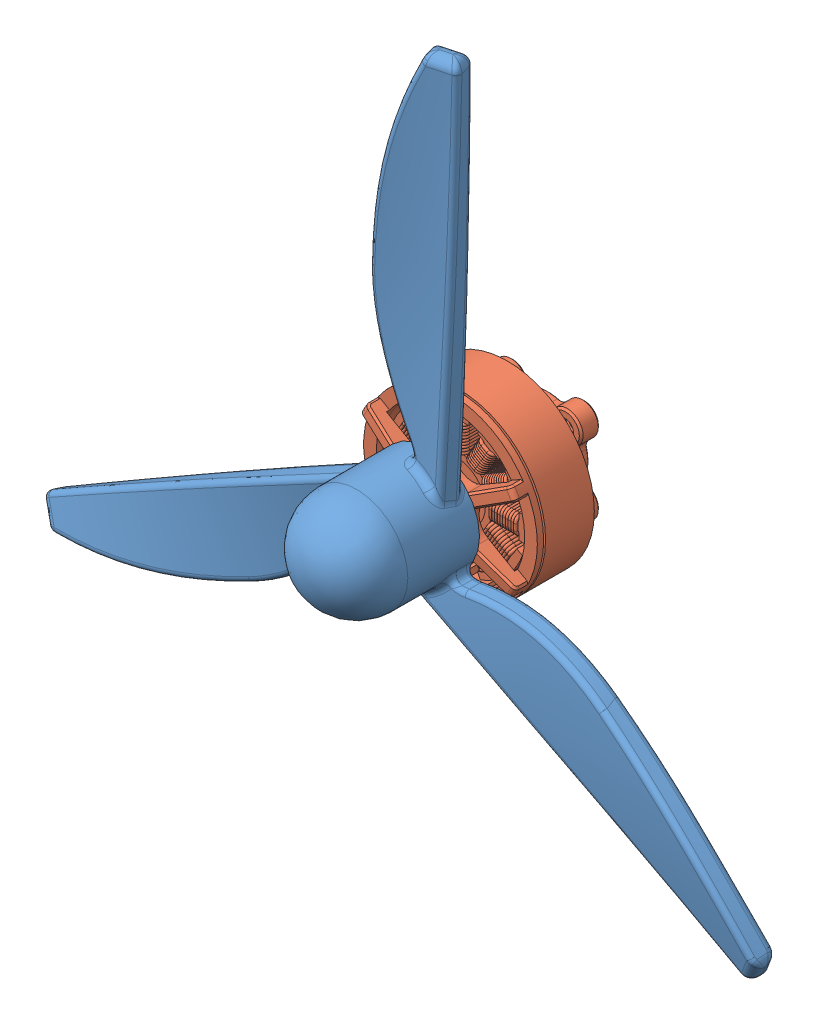
SolidWorks assembly 装配体3, configuration 默认. Lengths in mm.
Overall size (116.58 102.47 38.52).
2 component instances, 2 part files, 2 mates.
Components (placement in the parent):
- 螺旋桨-1: 螺旋桨 [Default] at (-26.4423 4.6884 108.4767) size (116.58 102.47 22.65)
- 2207电机-1: 2207电机 [默认] at (-26.4423 4.6884 88.8767) size (27.45 27.5 32.14)
Mates (geometry in assembly coordinates):
- 同心1: concentric: circle of 螺旋桨-1; circle of 2207电机-1
- 重合1: coincident anti-aligned: plane of 螺旋桨-1 through (-26.4423 4.6884 108.4767) normal (0 0 -1); plane of 2207电机-1 through (-26.4423 4.6884 108.4767) normal (0 0 1)
